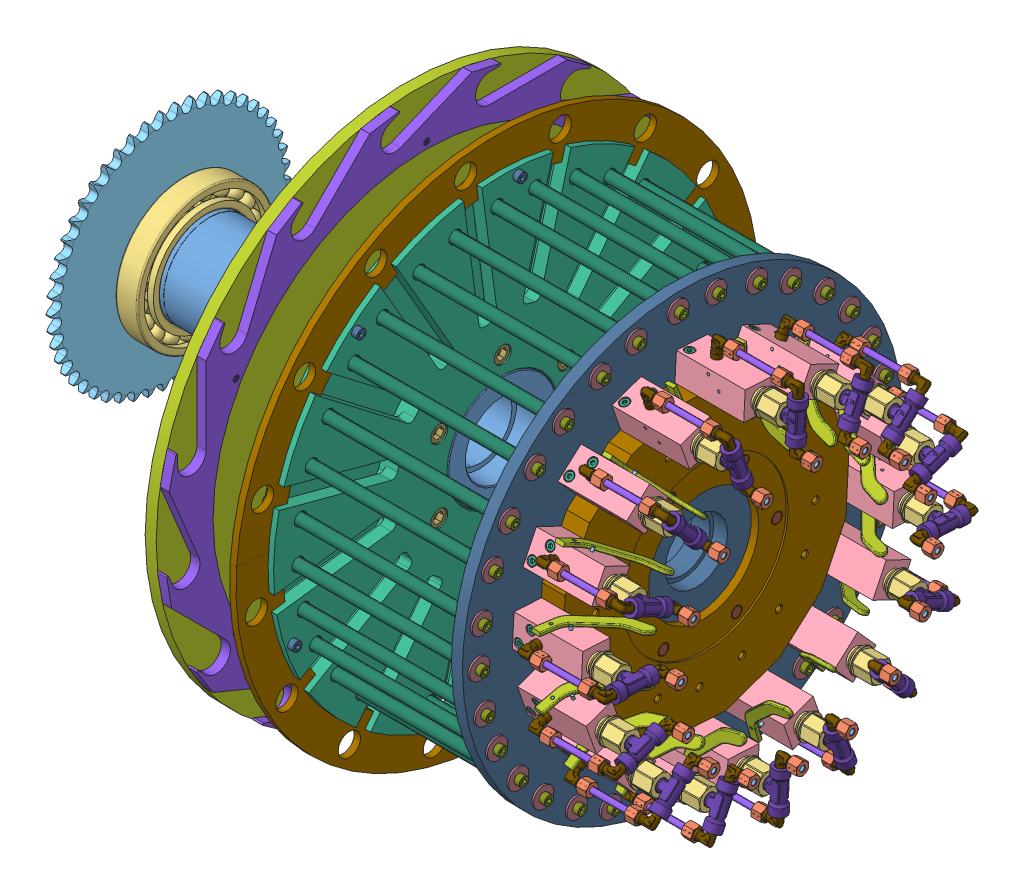
SolidWorks assembly assieme parte rotante, configuration Default. Lengths in mm.
Overall size (749.63 778.63 778.63).
555 component instances, 28 part files, 77 mates.
Components (placement in the parent):
- albero rotazione piatti-1: albero rotazione piatti [Default] at (60.413 18.3637 415) size (415 200 200)
- seger 100mm-1: seger 100mm [KS 1336 E - 100] at (-146.4567 18.3637 415) x (0 0 -1) z (1 0 0) size (107.55 112.98 3)
- SKF - 6020 - 20,DE,NC,20_68-1: SKF - 6020 - 20,DE,NC,20_68 [SKF - 6020 - 20,DE,NC,20_68] at (-131.4567 18.3637 415) x (1 0 0) z (0 -0.434476 -0.900684) size (24 150 150)
- calettatore d95-1: calettatore d95 [Default] at (-178.8867 18.3637 415) size (39.5 135 135)
- Chain wheel ISO - 50Z 10A-1-1: Chain wheel ISO - 50Z 10A-1 [Chain wheel ISO - 50Z 10A-1 --50SB120H25L95.0N] at (-164.8867 18.3637 415) size (25 262.06 262.51)
- Disco supporto montaggio e Colonne-1: Disco supporto montaggio e Colonne [Default] at (204.0433 18.3637 415) x (0 -0.866025 -0.5) z (1 0 0) size (499.6 499.6 29)
- SKF - 6020 - 20,DE,NC,20_68-2: SKF - 6020 - 20,DE,NC,20_68 [SKF - 6020 - 20,DE,NC,20_68] at (62.0433 18.3637 415) x (1 0 0) z (0 -0.432628 -0.901573) size (24 150 150)
- piatto rotante porta tappi-1: piatto rotante porta tappi [Default] at (99.0433 18.3637 415) x (0 0 -1) z (1 0 0) size (570 570 20.57)
- disco trasportatore tappi 31-1: disco trasportatore tappi 31 [Default] at (111.0433 18.3637 415) x (0 0.5 -0.866025) z (1 0 0) size (570 570 10.42)
- Distributore Rotante-1: Distributore Rotante [Default] at (425.0433 18.3637 415) x (0 -0.055301 -0.99847) z (1 0 0) size (310 310 25.54)
- disco trascinato porta distributore vuoto-1: disco trascinato porta distributore vuoto [Default] at (400.0433 18.3637 415) x (0 0.055301 0.99847) z (-1 0 0) size (480 480 50)
- m12 35mm-1: m12 35mm [ISO 4762 M12 x 35 - 35N] at (376.0433 -53.0243 378.8925) x (1 0 0) z (0 -0.5 0.866025) size (47 18 18)
- m12 90mm-3: m12 90mm [ISO 4762 M12 x 90 - 90N] at (203.0433 -21.6363 345.718) x (-1 0 0) z (0 -0.5 0.866025) size (102 18 18)
- rondella m6 22mm-1: rondella m6 22mm [Washer ISO 7094 - 6] at (99.0433 -101.6363 207.1539) x (1 0 0) z (0 -1 0) size (2 22 22)
- M6 20mm-1: M6 20mm [ISO 4762 M6 x 20 - 20N] at (91.0433 -101.6363 207.1539) x (1 0 0) z (0 0.5 0.866025) size (26 10 10)
- m12 35mm-2: m12 35mm [ISO 4762 M12 x 35 - 35N] at (376.0433 13.9397 335.1224) x (1 0 0) z (0 -1 0) size (47 18 18)
- m12 35mm-3: m12 35mm [ISO 4762 M12 x 35 - 35N] at (376.0433 85.3277 371.2299) x (1 0 0) z (0 -0.5 -0.866025) size (47 18 18)
- m12 35mm-4: m12 35mm [ISO 4762 M12 x 35 - 35N] at (376.0433 89.7517 451.1075) x (1 0 0) z (0 0.5 -0.866025) size (47 18 18)
- m12 35mm-5: m12 35mm [ISO 4762 M12 x 35 - 35N] at (376.0433 22.7877 494.8776) x (1 0 0) z (0 1 0) size (47 18 18)
- m12 35mm-6: m12 35mm [ISO 4762 M12 x 35 - 35N] at (376.0433 -48.6003 458.7701) x (1 0 0) z (0 0.5 0.866025) size (47 18 18)
- rondella m6 22mm-2: rondella m6 22mm [Washer ISO 7094 - 6] at (99.0433 138.3637 207.1539) x (1 0 0) z (0 -0.5 -0.866025) size (2 22 22)
- rondella m6 22mm-3: rondella m6 22mm [Washer ISO 7094 - 6] at (99.0433 258.3637 415) x (1 0 0) z (0 0.5 -0.866025) size (2 22 22)
- rondella m6 22mm-4: rondella m6 22mm [Washer ISO 7094 - 6] at (99.0433 138.3637 622.8461) x (1 0 0) z (0 1 0) size (2 22 22)
- rondella m6 22mm-5: rondella m6 22mm [Washer ISO 7094 - 6] at (99.0433 -101.6363 622.8461) x (1 0 0) z (0 0.5 0.866025) size (2 22 22)
- rondella m6 22mm-6: rondella m6 22mm [Washer ISO 7094 - 6] at (99.0433 -221.6363 415) x (1 0 0) z (0 -0.5 0.866025) size (2 22 22)
- M6 20mm-2: M6 20mm [ISO 4762 M6 x 20 - 20N] at (91.0433 138.3637 207.1539) x (1 0 0) z (0 -0.5 0.866025) size (26 10 10)
- M6 20mm-3: M6 20mm [ISO 4762 M6 x 20 - 20N] at (91.0433 258.3637 415) x (1 0 0) z (0 -1 0) size (26 10 10)
- M6 20mm-4: M6 20mm [ISO 4762 M6 x 20 - 20N] at (91.0433 138.3637 622.8461) x (1 0 0) z (0 -0.5 -0.866025) size (26 10 10)
- M6 20mm-5: M6 20mm [ISO 4762 M6 x 20 - 20N] at (91.0433 -101.6363 622.8461) x (1 0 0) z (0 0.5 -0.866025) size (26 10 10)
- M6 20mm-6: M6 20mm [ISO 4762 M6 x 20 - 20N] at (91.0433 -221.6363 415) x (1 0 0) z (0 1 0) size (26 10 10)
- m12 90mm-4: m12 90mm [ISO 4762 M12 x 90 - 90N] at (203.0433 58.3637 345.718) x (-1 0 0) z (0 -1 0) size (102 18 18)
- m12 90mm-5: m12 90mm [ISO 4762 M12 x 90 - 90N] at (203.0433 98.3637 415) x (-1 0 0) z (0 -0.5 -0.866025) size (102 18 18)
- m12 90mm-6: m12 90mm [ISO 4762 M12 x 90 - 90N] at (203.0433 58.3637 484.282) x (-1 0 0) z (0 0.5 -0.866025) size (102 18 18)
- m12 90mm-7: m12 90mm [ISO 4762 M12 x 90 - 90N] at (203.0433 -21.6363 484.282) x (-1 0 0) z (0 1 0) size (102 18 18)
- m12 90mm-8: m12 90mm [ISO 4762 M12 x 90 - 90N] at (203.0433 -61.6363 415) x (-1 0 0) z (0 0.5 0.866025) size (102 18 18)
- asta scorrimento carello-1: asta scorrimento carello [Default] at (287.5433 70.1437 197.9013) x (0 0 -1) z (1 0 0) size (12 12 225)
- rondella m6 22mm-7: rondella m6 22mm [Washer ISO 7094 - 6] at (175.0433 70.1437 197.9013) x (1 0 0) z (0 -1 0) size (2 22 22)
- M6 16mm-1: M6 16mm [ISO 4762 M6 x 16 - 16N] at (167.0433 70.1437 197.9013) size (22 10 10)
- M6 16mm-2: M6 16mm [ISO 4762 M6 x 16 - 16N] at (408.0433 70.1437 197.9013) x (-1 0 0) z (0 0 -1) size (22 10 10)
- rondella m6 22mm-8: rondella m6 22mm [Washer ISO 7094 - 6] at (400.0433 70.1437 197.9013) x (-1 0 0) z (0 1 0) size (2 22 22)
- rondella m6 22mm-9: rondella m6 22mm [Washer ISO 7094 - 6] at (175.0433 24.5373 191.8971) x (1 0 0) z (0 -0.965926 -0.258819) size (2 22 22)
- M6 16mm-3: M6 16mm [ISO 4762 M6 x 16 - 16N] at (167.0433 24.5373 191.8971) x (1 0 0) z (0 0.258819 -0.965926) size (22 10 10)
- asta scorrimento carello-2: asta scorrimento carello [Default] at (287.5433 24.5373 191.8971) x (0 0.258819 -0.965926) z (-1 0 0) size (12 12 225)
- rondella m6 22mm-10: rondella m6 22mm [Washer ISO 7094 - 6] at (400.0433 24.5373 191.8971) x (-1 0 0) z (0 0.965926 0.258819) size (2 22 22)
- M6 16mm-4: M6 16mm [ISO 4762 M6 x 16 - 16N] at (408.0433 24.5373 191.8971) x (-1 0 0) z (0 -0.258819 0.965926) size (22 10 10)
- AssiemeValvola-1: AssiemeValvola [Default] at (515.3257 74.6348 254.5832) x (0 -0.331007 0.943628) z (0 0.943628 0.331007) size (90.26 138.63 38)
  - RaccordoT-1: RaccordoT [Default] at origin size (43 29.75 16.5)
  - Raccordo a L-1: Raccordo a L [Default] at (-30 0 0) x (0 -1 0) z (0 0 -1) size (28.34 25.51 14.01)
    - 1809_06_10_01-1: 1809_06_10_01 [Default] at origin size (22.49 23 10)
    - 1809_06_10_02-1: 1809_06_10_02 [Default] at origin size (6.5 8.5 8.5)
    - 1809_06_10_03-1: 1809_06_10_03 [Default] at origin size (11.02 15.01 14.01)
  - Raccordo a L-2: Raccordo a L [Default] at (30 0 0) x (0 1 0) z (0 0 -1) size (28.34 25.51 14.01)
    - 1809_06_10_01-1: 1809_06_10_01 [Default] at origin size (22.49 23 10)
    - 1809_06_10_02-1: 1809_06_10_02 [Default] at origin size (6.5 8.5 8.5)
    - 1809_06_10_03-1: 1809_06_10_03 [Default] at origin size (11.02 15.01 14.01)
  - TappoChiusura-1: TappoChiusura [Default] at (0 -32 0) x (0 -1 0) z (0 0 1) size (38.28 26.74 26.74)
  - CorpoValvola-1: CorpoValvola [Default] at (-15 -115.2824 0) size (30 75 34)
  - Raccordo a L-3: Raccordo a L [Default] at (-30 -88.2824 0) x (0 1 0) z (0 0 1) size (28.34 25.51 14.01)
    - 1809_06_10_01-1: 1809_06_10_01 [Default] at origin size (22.49 23 10)
    - 1809_06_10_02-1: 1809_06_10_02 [Default] at origin size (6.5 8.5 8.5)
    - 1809_06_10_03-1: 1809_06_10_03 [Default] at origin size (11.02 15.01 14.01)
  - Spina_3x38-1: Spina_3x38 [Default] at (0 -68.2824 -21) x (-1 0 0) z (0 0 1) size (3 3 38)
  - Spina_3x38-2: Spina_3x38 [Default] at (-10 -80.2824 -21) x (0.996193 0.087174 0) z (0 0 1) size (3 3 38)
  - M5 40mm-3: M5 40mm [ISO 4762 M5 x 40 - 40N] at (-14.6 -108.7824 9) size (45 8.5 8.5)
  - M5 40mm-2: M5 40mm [ISO 4762 M5 x 40 - 40N] at (-14.6 -96.7824 -9) size (45 8.5 8.5)
  - LevaValvola-1: LevaValvola [Default] at (-24.507 -86.571 -17) x (0.996193 0.087174 0) z (0 0 1) size (77.55 60.2 4)
  - Tubo-1: Tubo [Default] at (-30 -15.9665 0) x (1 0 0) z (0 -1 0) size (6 6 56.4)
- M6 16mm-5: M6 16mm [ISO 4762 M6 x 16 - 16N] at (167.0433 -16.8778 194.6116) x (1 0 0) z (0 0.382683 0.92388) size (22 10 10)
- M6 16mm-6: M6 16mm [ISO 4762 M6 x 16 - 16N] at (167.0433 -98.5342 224.874) x (1 0 0) z (0 0.707107 0.707107) size (22 10 10)
- M6 16mm-7: M6 16mm [ISO 4762 M6 x 16 - 16N] at (167.0433 -162.3939 284.0814) x (1 0 0) z (0 0.92388 0.382683) size (22 10 10)
- M6 16mm-8: M6 16mm [ISO 4762 M6 x 16 - 16N] at (167.0433 -198.735 363.22) x (1 0 0) z (0 1 0) size (22 10 10)
- M6 16mm-9: M6 16mm [ISO 4762 M6 x 16 - 16N] at (167.0433 -202.0247 450.2415) x (1 0 0) z (0 0.92388 -0.382683) size (22 10 10)
- M6 16mm-10: M6 16mm [ISO 4762 M6 x 16 - 16N] at (167.0433 -171.7623 531.8979) x (1 0 0) z (0 0.707107 -0.707107) size (22 10 10)
- M6 16mm-11: M6 16mm [ISO 4762 M6 x 16 - 16N] at (167.0433 -112.5549 595.7576) x (1 0 0) z (0 0.382683 -0.92388) size (22 10 10)
- M6 16mm-12: M6 16mm [ISO 4762 M6 x 16 - 16N] at (167.0433 -33.4163 632.0987) x (1 0 0) z (0 0 -1) size (22 10 10)
- M6 16mm-13: M6 16mm [ISO 4762 M6 x 16 - 16N] at (167.0433 53.6052 635.3884) x (1 0 0) z (0 -0.382683 -0.92388) size (22 10 10)
- M6 16mm-14: M6 16mm [ISO 4762 M6 x 16 - 16N] at (167.0433 135.2616 605.126) x (1 0 0) z (0 -0.707107 -0.707107) size (22 10 10)
- M6 16mm-15: M6 16mm [ISO 4762 M6 x 16 - 16N] at (167.0433 199.1213 545.9186) x (1 0 0) z (0 -0.92388 -0.382683) size (22 10 10)
- M6 16mm-16: M6 16mm [ISO 4762 M6 x 16 - 16N] at (167.0433 235.4624 466.78) x (1 0 0) z (0 -1 0) size (22 10 10)
- M6 16mm-17: M6 16mm [ISO 4762 M6 x 16 - 16N] at (167.0433 238.7521 379.7585) x (1 0 0) z (0 -0.92388 0.382683) size (22 10 10)
- M6 16mm-18: M6 16mm [ISO 4762 M6 x 16 - 16N] at (167.0433 208.4897 298.1021) x (1 0 0) z (0 -0.707107 0.707107) size (22 10 10)
- M6 16mm-19: M6 16mm [ISO 4762 M6 x 16 - 16N] at (167.0433 149.2823 234.2424) x (1 0 0) z (0 -0.382683 0.92388) size (22 10 10)
- rondella m6 22mm-11: rondella m6 22mm [Washer ISO 7094 - 6] at (175.0433 -16.8778 194.6116) x (1 0 0) z (0 -0.92388 0.382683) size (2 22 22)
- rondella m6 22mm-12: rondella m6 22mm [Washer ISO 7094 - 6] at (175.0433 -98.5342 224.874) x (1 0 0) z (0 -0.707107 0.707107) size (2 22 22)
- rondella m6 22mm-13: rondella m6 22mm [Washer ISO 7094 - 6] at (175.0433 -162.3939 284.0814) x (1 0 0) z (0 -0.382683 0.92388) size (2 22 22)
- rondella m6 22mm-14: rondella m6 22mm [Washer ISO 7094 - 6] at (175.0433 -198.735 363.22) size (2 22 22)
- rondella m6 22mm-15: rondella m6 22mm [Washer ISO 7094 - 6] at (175.0433 -202.0247 450.2415) x (1 0 0) z (0 0.382683 0.92388) size (2 22 22)
- rondella m6 22mm-16: rondella m6 22mm [Washer ISO 7094 - 6] at (175.0433 -171.7623 531.8979) x (1 0 0) z (0 0.707107 0.707107) size (2 22 22)
- rondella m6 22mm-17: rondella m6 22mm [Washer ISO 7094 - 6] at (175.0433 -112.5549 595.7576) x (1 0 0) z (0 0.92388 0.382683) size (2 22 22)
- rondella m6 22mm-18: rondella m6 22mm [Washer ISO 7094 - 6] at (175.0433 -33.4163 632.0987) x (1 0 0) z (0 1 0) size (2 22 22)
- rondella m6 22mm-19: rondella m6 22mm [Washer ISO 7094 - 6] at (175.0433 53.6052 635.3884) x (1 0 0) z (0 0.92388 -0.382683) size (2 22 22)
- rondella m6 22mm-20: rondella m6 22mm [Washer ISO 7094 - 6] at (175.0433 135.2616 605.126) x (1 0 0) z (0 0.707107 -0.707107) size (2 22 22)
- rondella m6 22mm-21: rondella m6 22mm [Washer ISO 7094 - 6] at (175.0433 199.1213 545.9186) x (1 0 0) z (0 0.382683 -0.92388) size (2 22 22)
- rondella m6 22mm-22: rondella m6 22mm [Washer ISO 7094 - 6] at (175.0433 235.4624 466.78) x (1 0 0) z (0 0 -1) size (2 22 22)
- rondella m6 22mm-23: rondella m6 22mm [Washer ISO 7094 - 6] at (175.0433 238.7521 379.7585) x (1 0 0) z (0 -0.382683 -0.92388) size (2 22 22)
- rondella m6 22mm-24: rondella m6 22mm [Washer ISO 7094 - 6] at (175.0433 208.4897 298.1021) x (1 0 0) z (0 -0.707107 -0.707107) size (2 22 22)
- rondella m6 22mm-25: rondella m6 22mm [Washer ISO 7094 - 6] at (175.0433 149.2823 234.2424) x (1 0 0) z (0 -0.92388 -0.382683) size (2 22 22)
- asta scorrimento carello-3: asta scorrimento carello [Default] at (287.5433 -16.8778 194.6116) x (0 -0.382683 -0.92388) z (1 0 0) size (12 12 225)
- asta scorrimento carello-4: asta scorrimento carello [Default] at (287.5433 -98.5342 224.874) x (0 -0.707107 -0.707107) z (1 0 0) size (12 12 225)
- asta scorrimento carello-5: asta scorrimento carello [Default] at (287.5433 -162.3939 284.0814) x (0 -0.92388 -0.382683) z (1 0 0) size (12 12 225)
- asta scorrimento carello-6: asta scorrimento carello [Default] at (287.5433 -198.735 363.22) x (0 -1 0) z (1 0 0) size (12 12 225)
- asta scorrimento carello-7: asta scorrimento carello [Default] at (287.5433 -202.0247 450.2415) x (0 -0.92388 0.382683) z (1 0 0) size (12 12 225)
- asta scorrimento carello-8: asta scorrimento carello [Default] at (287.5433 -171.7623 531.8979) x (0 -0.707107 0.707107) z (1 0 0) size (12 12 225)
- asta scorrimento carello-9: asta scorrimento carello [Default] at (287.5433 -112.5549 595.7576) x (0 -0.382683 0.92388) z (1 0 0) size (12 12 225)
- asta scorrimento carello-10: asta scorrimento carello [Default] at (287.5433 -33.4163 632.0987) x (0 0 1) z (1 0 0) size (12 12 225)
- asta scorrimento carello-11: asta scorrimento carello [Default] at (287.5433 53.6052 635.3884) x (0 0.382683 0.92388) z (1 0 0) size (12 12 225)
- asta scorrimento carello-12: asta scorrimento carello [Default] at (287.5433 135.2616 605.126) x (0 0.707107 0.707107) z (1 0 0) size (12 12 225)
- asta scorrimento carello-13: asta scorrimento carello [Default] at (287.5433 199.1213 545.9186) x (0 0.92388 0.382683) z (1 0 0) size (12 12 225)
- asta scorrimento carello-14: asta scorrimento carello [Default] at (287.5433 235.4624 466.78) x (0 1 0) z (1 0 0) size (12 12 225)
- asta scorrimento carello-15: asta scorrimento carello [Default] at (287.5433 238.7521 379.7585) x (0 0.92388 -0.382683) z (1 0 0) size (12 12 225)
- asta scorrimento carello-16: asta scorrimento carello [Default] at (287.5433 208.4897 298.1021) x (0 0.707107 -0.707107) z (1 0 0) size (12 12 225)
- asta scorrimento carello-17: asta scorrimento carello [Default] at (287.5433 149.2823 234.2424) x (0 0.382683 -0.92388) z (1 0 0) size (12 12 225)
- M6 16mm-20: M6 16mm [ISO 4762 M6 x 16 - 16N] at (408.0433 -16.8778 194.6116) x (-1 0 0) z (0 -0.382683 -0.92388) size (22 10 10)
- M6 16mm-21: M6 16mm [ISO 4762 M6 x 16 - 16N] at (408.0433 -98.5342 224.874) x (-1 0 0) z (0 -0.707107 -0.707107) size (22 10 10)
- M6 16mm-22: M6 16mm [ISO 4762 M6 x 16 - 16N] at (408.0433 -162.3939 284.0814) x (-1 0 0) z (0 -0.92388 -0.382683) size (22 10 10)
- M6 16mm-23: M6 16mm [ISO 4762 M6 x 16 - 16N] at (408.0433 -198.735 363.22) x (-1 0 0) z (0 -1 0) size (22 10 10)
- M6 16mm-24: M6 16mm [ISO 4762 M6 x 16 - 16N] at (408.0433 -202.0247 450.2415) x (-1 0 0) z (0 -0.92388 0.382683) size (22 10 10)
- M6 16mm-25: M6 16mm [ISO 4762 M6 x 16 - 16N] at (408.0433 -171.7623 531.8979) x (-1 0 0) z (0 -0.707107 0.707107) size (22 10 10)
- M6 16mm-26: M6 16mm [ISO 4762 M6 x 16 - 16N] at (408.0433 -112.5549 595.7576) x (-1 0 0) z (0 -0.382683 0.92388) size (22 10 10)
- M6 16mm-27: M6 16mm [ISO 4762 M6 x 16 - 16N] at (408.0433 -33.4163 632.0987) x (-1 0 0) z (0 0 1) size (22 10 10)
- M6 16mm-28: M6 16mm [ISO 4762 M6 x 16 - 16N] at (408.0433 53.6052 635.3884) x (-1 0 0) z (0 0.382683 0.92388) size (22 10 10)
- M6 16mm-29: M6 16mm [ISO 4762 M6 x 16 - 16N] at (408.0433 135.2616 605.126) x (-1 0 0) z (0 0.707107 0.707107) size (22 10 10)
- M6 16mm-30: M6 16mm [ISO 4762 M6 x 16 - 16N] at (408.0433 199.1213 545.9186) x (-1 0 0) z (0 0.92388 0.382683) size (22 10 10)
- M6 16mm-31: M6 16mm [ISO 4762 M6 x 16 - 16N] at (408.0433 235.4624 466.78) x (-1 0 0) z (0 1 0) size (22 10 10)
- M6 16mm-32: M6 16mm [ISO 4762 M6 x 16 - 16N] at (408.0433 238.7521 379.7585) x (-1 0 0) z (0 0.92388 -0.382683) size (22 10 10)
- M6 16mm-33: M6 16mm [ISO 4762 M6 x 16 - 16N] at (408.0433 208.4897 298.1021) x (-1 0 0) z (0 0.707107 -0.707107) size (22 10 10)
- M6 16mm-34: M6 16mm [ISO 4762 M6 x 16 - 16N] at (408.0433 149.2823 234.2424) x (-1 0 0) z (0 0.382683 -0.92388) size (22 10 10)
- rondella m6 22mm-26: rondella m6 22mm [Washer ISO 7094 - 6] at (400.0433 -16.8778 194.6116) x (-1 0 0) z (0 0.92388 -0.382683) size (2 22 22)
- rondella m6 22mm-27: rondella m6 22mm [Washer ISO 7094 - 6] at (400.0433 -98.5342 224.874) x (-1 0 0) z (0 0.707107 -0.707107) size (2 22 22)
- rondella m6 22mm-28: rondella m6 22mm [Washer ISO 7094 - 6] at (400.0433 -162.3939 284.0814) x (-1 0 0) z (0 0.382683 -0.92388) size (2 22 22)
- rondella m6 22mm-29: rondella m6 22mm [Washer ISO 7094 - 6] at (400.0433 -198.735 363.22) x (-1 0 0) z (0 0 -1) size (2 22 22)
- rondella m6 22mm-30: rondella m6 22mm [Washer ISO 7094 - 6] at (400.0433 -202.0247 450.2415) x (-1 0 0) z (0 -0.382683 -0.92388) size (2 22 22)
- rondella m6 22mm-31: rondella m6 22mm [Washer ISO 7094 - 6] at (400.0433 -171.7623 531.8979) x (-1 0 0) z (0 -0.707107 -0.707107) size (2 22 22)
- rondella m6 22mm-32: rondella m6 22mm [Washer ISO 7094 - 6] at (400.0433 -112.5549 595.7576) x (-1 0 0) z (0 -0.92388 -0.382683) size (2 22 22)
- rondella m6 22mm-33: rondella m6 22mm [Washer ISO 7094 - 6] at (400.0433 -33.4163 632.0987) x (-1 0 0) z (0 -1 0) size (2 22 22)
- rondella m6 22mm-34: rondella m6 22mm [Washer ISO 7094 - 6] at (400.0433 53.6052 635.3884) x (-1 0 0) z (0 -0.92388 0.382683) size (2 22 22)
- rondella m6 22mm-35: rondella m6 22mm [Washer ISO 7094 - 6] at (400.0433 135.2616 605.126) x (-1 0 0) z (0 -0.707107 0.707107) size (2 22 22)
- rondella m6 22mm-36: rondella m6 22mm [Washer ISO 7094 - 6] at (400.0433 199.1213 545.9186) x (-1 0 0) z (0 -0.382683 0.92388) size (2 22 22)
- rondella m6 22mm-37: rondella m6 22mm [Washer ISO 7094 - 6] at (400.0433 235.4624 466.78) x (-1 0 0) z (0 0 1) size (2 22 22)
- rondella m6 22mm-38: rondella m6 22mm [Washer ISO 7094 - 6] at (400.0433 238.7521 379.7585) x (-1 0 0) z (0 0.382683 0.92388) size (2 22 22)
- rondella m6 22mm-39: rondella m6 22mm [Washer ISO 7094 - 6] at (400.0433 208.4897 298.1021) x (-1 0 0) z (0 0.707107 0.707107) size (2 22 22)
- rondella m6 22mm-40: rondella m6 22mm [Washer ISO 7094 - 6] at (400.0433 149.2823 234.2424) x (-1 0 0) z (0 0.92388 0.382683) size (2 22 22)
- rondella m6 22mm-41: rondella m6 22mm [Washer ISO 7094 - 6] at (175.0433 -61.3104 206.5173) x (1 0 0) z (0 -0.991445 0.130526) size (2 22 22)
- rondella m6 22mm-42: rondella m6 22mm [Washer ISO 7094 - 6] at (175.0433 -135.0285 252.8771) x (1 0 0) z (0 -0.866025 0.5) size (2 22 22)
- rondella m6 22mm-43: rondella m6 22mm [Washer ISO 7094 - 6] at (175.0433 -185.3939 323.9186) x (1 0 0) z (0 -0.608761 0.793353) size (2 22 22)
- rondella m6 22mm-44: rondella m6 22mm [Washer ISO 7094 - 6] at (175.0433 -204.7392 408.8264) x (1 0 0) z (0 -0.258819 0.965926) size (2 22 22)
- rondella m6 22mm-45: rondella m6 22mm [Washer ISO 7094 - 6] at (175.0433 -190.119 494.6741) x (1 0 0) z (0 0.130526 0.991445) size (2 22 22)
- rondella m6 22mm-46: rondella m6 22mm [Washer ISO 7094 - 6] at (175.0433 -143.7592 568.3922) x (1 0 0) z (0 0.5 0.866025) size (2 22 22)
- rondella m6 22mm-47: rondella m6 22mm [Washer ISO 7094 - 6] at (175.0433 -72.7177 618.7576) x (1 0 0) z (0 0.793353 0.608761) size (2 22 22)
- rondella m6 22mm-48: rondella m6 22mm [Washer ISO 7094 - 6] at (175.0433 12.1901 638.1029) x (1 0 0) z (0 0.965926 0.258819) size (2 22 22)
- rondella m6 22mm-49: rondella m6 22mm [Washer ISO 7094 - 6] at (175.0433 98.0378 623.4827) x (1 0 0) z (0 0.991445 -0.130526) size (2 22 22)
- rondella m6 22mm-50: rondella m6 22mm [Washer ISO 7094 - 6] at (175.0433 171.7559 577.1229) x (1 0 0) z (0 0.866025 -0.5) size (2 22 22)
- rondella m6 22mm-51: rondella m6 22mm [Washer ISO 7094 - 6] at (175.0433 222.1213 506.0814) x (1 0 0) z (0 0.608761 -0.793353) size (2 22 22)
- rondella m6 22mm-52: rondella m6 22mm [Washer ISO 7094 - 6] at (175.0433 241.4666 421.1736) x (1 0 0) z (0 0.258819 -0.965926) size (2 22 22)
- rondella m6 22mm-53: rondella m6 22mm [Washer ISO 7094 - 6] at (175.0433 226.8464 335.3259) x (1 0 0) z (0 -0.130526 -0.991445) size (2 22 22)
- rondella m6 22mm-54: rondella m6 22mm [Washer ISO 7094 - 6] at (175.0433 180.4866 261.6078) x (1 0 0) z (0 -0.5 -0.866025) size (2 22 22)
- rondella m6 22mm-55: rondella m6 22mm [Washer ISO 7094 - 6] at (175.0433 109.4451 211.2424) x (1 0 0) z (0 -0.793353 -0.608761) size (2 22 22)
- M6 16mm-35: M6 16mm [ISO 4762 M6 x 16 - 16N] at (167.0433 -61.3104 206.5173) x (1 0 0) z (0 -0.130526 -0.991445) size (22 10 10)
- M6 16mm-36: M6 16mm [ISO 4762 M6 x 16 - 16N] at (167.0433 -135.0285 252.8771) x (1 0 0) z (0 -0.5 -0.866025) size (22 10 10)
- M6 16mm-37: M6 16mm [ISO 4762 M6 x 16 - 16N] at (167.0433 -185.3939 323.9186) x (1 0 0) z (0 -0.793353 -0.608761) size (22 10 10)
- M6 16mm-38: M6 16mm [ISO 4762 M6 x 16 - 16N] at (167.0433 -204.7392 408.8264) x (1 0 0) z (0 -0.965926 -0.258819) size (22 10 10)
- M6 16mm-39: M6 16mm [ISO 4762 M6 x 16 - 16N] at (167.0433 -190.119 494.6741) x (1 0 0) z (0 -0.991445 0.130526) size (22 10 10)
- M6 16mm-40: M6 16mm [ISO 4762 M6 x 16 - 16N] at (167.0433 -143.7592 568.3922) x (1 0 0) z (0 -0.866025 0.5) size (22 10 10)
- M6 16mm-41: M6 16mm [ISO 4762 M6 x 16 - 16N] at (167.0433 -72.7177 618.7576) x (1 0 0) z (0 -0.608761 0.793353) size (22 10 10)
- M6 16mm-42: M6 16mm [ISO 4762 M6 x 16 - 16N] at (167.0433 12.1901 638.1029) x (1 0 0) z (0 -0.258819 0.965926) size (22 10 10)
- M6 16mm-43: M6 16mm [ISO 4762 M6 x 16 - 16N] at (167.0433 98.0378 623.4827) x (1 0 0) z (0 0.130526 0.991445) size (22 10 10)
- M6 16mm-44: M6 16mm [ISO 4762 M6 x 16 - 16N] at (167.0433 171.7559 577.1229) x (1 0 0) z (0 0.5 0.866025) size (22 10 10)
- M6 16mm-45: M6 16mm [ISO 4762 M6 x 16 - 16N] at (167.0433 222.1213 506.0814) x (1 0 0) z (0 0.793353 0.608761) size (22 10 10)
- M6 16mm-46: M6 16mm [ISO 4762 M6 x 16 - 16N] at (167.0433 241.4666 421.1736) x (1 0 0) z (0 0.965926 0.258819) size (22 10 10)
- M6 16mm-47: M6 16mm [ISO 4762 M6 x 16 - 16N] at (167.0433 226.8464 335.3259) x (1 0 0) z (0 0.991445 -0.130526) size (22 10 10)
- M6 16mm-48: M6 16mm [ISO 4762 M6 x 16 - 16N] at (167.0433 180.4866 261.6078) x (1 0 0) z (0 0.866025 -0.5) size (22 10 10)
- M6 16mm-49: M6 16mm [ISO 4762 M6 x 16 - 16N] at (167.0433 109.4451 211.2424) x (1 0 0) z (0 0.608761 -0.793353) size (22 10 10)
- asta scorrimento carello-18: asta scorrimento carello [Default] at (287.5433 -61.3104 206.5173) x (0 -0.130526 -0.991445) z (-1 0 0) size (12 12 225)
- asta scorrimento carello-19: asta scorrimento carello [Default] at (287.5433 -135.0285 252.8771) x (0 -0.5 -0.866025) z (-1 0 0) size (12 12 225)
- asta scorrimento carello-20: asta scorrimento carello [Default] at (287.5433 -185.3939 323.9186) x (0 -0.793353 -0.608761) z (-1 0 0) size (12 12 225)
- asta scorrimento carello-21: asta scorrimento carello [Default] at (287.5433 -204.7392 408.8264) x (0 -0.965926 -0.258819) z (-1 0 0) size (12 12 225)
- asta scorrimento carello-22: asta scorrimento carello [Default] at (287.5433 -190.119 494.6741) x (0 -0.991445 0.130526) z (-1 0 0) size (12 12 225)
- asta scorrimento carello-23: asta scorrimento carello [Default] at (287.5433 -143.7592 568.3922) x (0 -0.866025 0.5) z (-1 0 0) size (12 12 225)
- asta scorrimento carello-24: asta scorrimento carello [Default] at (287.5433 -72.7177 618.7576) x (0 -0.608761 0.793353) z (-1 0 0) size (12 12 225)
- asta scorrimento carello-25: asta scorrimento carello [Default] at (287.5433 12.1901 638.1029) x (0 -0.258819 0.965926) z (-1 0 0) size (12 12 225)
- asta scorrimento carello-26: asta scorrimento carello [Default] at (287.5433 98.0378 623.4827) x (0 0.130526 0.991445) z (-1 0 0) size (12 12 225)
- asta scorrimento carello-27: asta scorrimento carello [Default] at (287.5433 171.7559 577.1229) x (0 0.5 0.866025) z (-1 0 0) size (12 12 225)
- asta scorrimento carello-28: asta scorrimento carello [Default] at (287.5433 222.1213 506.0814) x (0 0.793353 0.608761) z (-1 0 0) size (12 12 225)
- asta scorrimento carello-29: asta scorrimento carello [Default] at (287.5433 241.4666 421.1736) x (0 0.965926 0.258819) z (-1 0 0) size (12 12 225)
- asta scorrimento carello-30: asta scorrimento carello [Default] at (287.5433 226.8464 335.3259) x (0 0.991445 -0.130526) z (-1 0 0) size (12 12 225)
- asta scorrimento carello-31: asta scorrimento carello [Default] at (287.5433 180.4866 261.6078) x (0 0.866025 -0.5) z (-1 0 0) size (12 12 225)
- asta scorrimento carello-32: asta scorrimento carello [Default] at (287.5433 109.4451 211.2424) x (0 0.608761 -0.793353) z (-1 0 0) size (12 12 225)
- rondella m6 22mm-56: rondella m6 22mm [Washer ISO 7094 - 6] at (400.0433 -61.3104 206.5173) x (-1 0 0) z (0 0.991445 -0.130526) size (2 22 22)
- rondella m6 22mm-57: rondella m6 22mm [Washer ISO 7094 - 6] at (400.0433 -135.0285 252.8771) x (-1 0 0) z (0 0.866025 -0.5) size (2 22 22)
- rondella m6 22mm-58: rondella m6 22mm [Washer ISO 7094 - 6] at (400.0433 -185.3939 323.9186) x (-1 0 0) z (0 0.608761 -0.793353) size (2 22 22)
- rondella m6 22mm-59: rondella m6 22mm [Washer ISO 7094 - 6] at (400.0433 -204.7392 408.8264) x (-1 0 0) z (0 0.258819 -0.965926) size (2 22 22)
- rondella m6 22mm-60: rondella m6 22mm [Washer ISO 7094 - 6] at (400.0433 -190.119 494.6741) x (-1 0 0) z (0 -0.130526 -0.991445) size (2 22 22)
- rondella m6 22mm-61: rondella m6 22mm [Washer ISO 7094 - 6] at (400.0433 -143.7592 568.3922) x (-1 0 0) z (0 -0.5 -0.866025) size (2 22 22)
- rondella m6 22mm-62: rondella m6 22mm [Washer ISO 7094 - 6] at (400.0433 -72.7177 618.7576) x (-1 0 0) z (0 -0.793353 -0.608761) size (2 22 22)
- rondella m6 22mm-63: rondella m6 22mm [Washer ISO 7094 - 6] at (400.0433 12.1901 638.1029) x (-1 0 0) z (0 -0.965926 -0.258819) size (2 22 22)
- rondella m6 22mm-64: rondella m6 22mm [Washer ISO 7094 - 6] at (400.0433 98.0378 623.4827) x (-1 0 0) z (0 -0.991445 0.130526) size (2 22 22)
- rondella m6 22mm-65: rondella m6 22mm [Washer ISO 7094 - 6] at (400.0433 171.7559 577.1229) x (-1 0 0) z (0 -0.866025 0.5) size (2 22 22)
- rondella m6 22mm-66: rondella m6 22mm [Washer ISO 7094 - 6] at (400.0433 222.1213 506.0814) x (-1 0 0) z (0 -0.608761 0.793353) size (2 22 22)
- rondella m6 22mm-67: rondella m6 22mm [Washer ISO 7094 - 6] at (400.0433 241.4666 421.1736) x (-1 0 0) z (0 -0.258819 0.965926) size (2 22 22)
- rondella m6 22mm-68: rondella m6 22mm [Washer ISO 7094 - 6] at (400.0433 226.8464 335.3259) x (-1 0 0) z (0 0.130526 0.991445) size (2 22 22)
- rondella m6 22mm-69: rondella m6 22mm [Washer ISO 7094 - 6] at (400.0433 180.4866 261.6078) x (-1 0 0) z (0 0.5 0.866025) size (2 22 22)
- rondella m6 22mm-70: rondella m6 22mm [Washer ISO 7094 - 6] at (400.0433 109.4451 211.2424) x (-1 0 0) z (0 0.793353 0.608761) size (2 22 22)
- M6 16mm-50: M6 16mm [ISO 4762 M6 x 16 - 16N] at (408.0433 -61.3104 206.5173) x (-1 0 0) z (0 0.130526 0.991445) size (22 10 10)
- M6 16mm-51: M6 16mm [ISO 4762 M6 x 16 - 16N] at (408.0433 -135.0285 252.8771) x (-1 0 0) z (0 0.5 0.866025) size (22 10 10)
- M6 16mm-52: M6 16mm [ISO 4762 M6 x 16 - 16N] at (408.0433 -185.3939 323.9186) x (-1 0 0) z (0 0.793353 0.608761) size (22 10 10)
- M6 16mm-53: M6 16mm [ISO 4762 M6 x 16 - 16N] at (408.0433 -204.7392 408.8264) x (-1 0 0) z (0 0.965926 0.258819) size (22 10 10)
- M6 16mm-54: M6 16mm [ISO 4762 M6 x 16 - 16N] at (408.0433 -190.119 494.6741) x (-1 0 0) z (0 0.991445 -0.130526) size (22 10 10)
- M6 16mm-55: M6 16mm [ISO 4762 M6 x 16 - 16N] at (408.0433 -143.7592 568.3922) x (-1 0 0) z (0 0.866025 -0.5) size (22 10 10)
- M6 16mm-56: M6 16mm [ISO 4762 M6 x 16 - 16N] at (408.0433 -72.7177 618.7576) x (-1 0 0) z (0 0.608761 -0.793353) size (22 10 10)
- M6 16mm-57: M6 16mm [ISO 4762 M6 x 16 - 16N] at (408.0433 12.1901 638.1029) x (-1 0 0) z (0 0.258819 -0.965926) size (22 10 10)
- M6 16mm-58: M6 16mm [ISO 4762 M6 x 16 - 16N] at (408.0433 98.0378 623.4827) x (-1 0 0) z (0 -0.130526 -0.991445) size (22 10 10)
- M6 16mm-59: M6 16mm [ISO 4762 M6 x 16 - 16N] at (408.0433 171.7559 577.1229) x (-1 0 0) z (0 -0.5 -0.866025) size (22 10 10)
- M6 16mm-60: M6 16mm [ISO 4762 M6 x 16 - 16N] at (408.0433 222.1213 506.0814) x (-1 0 0) z (0 -0.793353 -0.608761) size (22 10 10)
- M6 16mm-61: M6 16mm [ISO 4762 M6 x 16 - 16N] at (408.0433 241.4666 421.1736) x (-1 0 0) z (0 -0.965926 -0.258819) size (22 10 10)
- M6 16mm-62: M6 16mm [ISO 4762 M6 x 16 - 16N] at (408.0433 226.8464 335.3259) x (-1 0 0) z (0 -0.991445 0.130526) size (22 10 10)
- M6 16mm-63: M6 16mm [ISO 4762 M6 x 16 - 16N] at (408.0433 180.4866 261.6078) x (-1 0 0) z (0 -0.866025 0.5) size (22 10 10)
- M6 16mm-64: M6 16mm [ISO 4762 M6 x 16 - 16N] at (408.0433 109.4451 211.2424) x (-1 0 0) z (0 -0.608761 0.793353) size (22 10 10)
- AssiemeValvola-2: AssiemeValvola [Default] at (515.3257 8.9626 245.2601) x (0 0.055301 0.99847) z (0 0.99847 -0.055301) size (90.26 138.63 38)
  - RaccordoT-1: RaccordoT [Default] at origin size (43 29.75 16.5)
  - Raccordo a L-1: Raccordo a L [Default] at (-30 0 0) x (0 -1 0) z (0 0 -1) size (28.34 25.51 14.01)
    - 1809_06_10_01-1: 1809_06_10_01 [Default] at origin size (22.49 23 10)
    - 1809_06_10_02-1: 1809_06_10_02 [Default] at origin size (6.5 8.5 8.5)
    - 1809_06_10_03-1: 1809_06_10_03 [Default] at origin size (11.02 15.01 14.01)
  - Raccordo a L-2: Raccordo a L [Default] at (30 0 0) x (0 1 0) z (0 0 -1) size (28.34 25.51 14.01)
    - 1809_06_10_01-1: 1809_06_10_01 [Default] at origin size (22.49 23 10)
    - 1809_06_10_02-1: 1809_06_10_02 [Default] at origin size (6.5 8.5 8.5)
    - 1809_06_10_03-1: 1809_06_10_03 [Default] at origin size (11.02 15.01 14.01)
  - TappoChiusura-1: TappoChiusura [Default] at (0 -32 0) x (0 -1 0) z (0 0 1) size (38.28 26.74 26.74)
  - CorpoValvola-1: CorpoValvola [Default] at (-15 -115.2824 0) size (30 75 34)
  - Raccordo a L-3: Raccordo a L [Default] at (-30 -88.2824 0) x (0 1 0) z (0 0 1) size (28.34 25.51 14.01)
    - 1809_06_10_01-1: 1809_06_10_01 [Default] at origin size (22.49 23 10)
    - 1809_06_10_02-1: 1809_06_10_02 [Default] at origin size (6.5 8.5 8.5)
    - 1809_06_10_03-1: 1809_06_10_03 [Default] at origin size (11.02 15.01 14.01)
  - Spina_3x38-1: Spina_3x38 [Default] at (0 -68.2824 -21) x (-1 0 0) z (0 0 1) size (3 3 38)
  - Spina_3x38-2: Spina_3x38 [Default] at (-10 -80.2824 -21) x (0.996193 0.087174 0) z (0 0 1) size (3 3 38)
  - M5 40mm-3: M5 40mm [ISO 4762 M5 x 40 - 40N] at (-14.6 -108.7824 9) size (45 8.5 8.5)
  - M5 40mm-2: M5 40mm [ISO 4762 M5 x 40 - 40N] at (-14.6 -96.7824 -9) size (45 8.5 8.5)
  - LevaValvola-1: LevaValvola [Default] at (-24.507 -86.571 -17) x (0.996193 0.087174 0) z (0 0 1) size (77.55 60.2 4)
  - Tubo-1: Tubo [Default] at (-30 -15.9665 0) x (1 0 0) z (0 -1 0) size (6 6 56.4)
- AssiemeValvola-3: AssiemeValvola [Default] at (515.3257 -55.2784 261.7785) x (0 0.433189 0.901303) z (0 0.901303 -0.433189) size (90.26 138.63 38)
  - RaccordoT-1: RaccordoT [Default] at origin size (43 29.75 16.5)
  - Raccordo a L-1: Raccordo a L [Default] at (-30 0 0) x (0 -1 0) z (0 0 -1) size (28.34 25.51 14.01)
    - 1809_06_10_01-1: 1809_06_10_01 [Default] at origin size (22.49 23 10)
    - 1809_06_10_02-1: 1809_06_10_02 [Default] at origin size (6.5 8.5 8.5)
    - 1809_06_10_03-1: 1809_06_10_03 [Default] at origin size (11.02 15.01 14.01)
  - Raccordo a L-2: Raccordo a L [Default] at (30 0 0) x (0 1 0) z (0 0 -1) size (28.34 25.51 14.01)
    - 1809_06_10_01-1: 1809_06_10_01 [Default] at origin size (22.49 23 10)
    - 1809_06_10_02-1: 1809_06_10_02 [Default] at origin size (6.5 8.5 8.5)
    - 1809_06_10_03-1: 1809_06_10_03 [Default] at origin size (11.02 15.01 14.01)
  - TappoChiusura-1: TappoChiusura [Default] at (0 -32 0) x (0 -1 0) z (0 0 1) size (38.28 26.74 26.74)
  - CorpoValvola-1: CorpoValvola [Default] at (-15 -115.2824 0) size (30 75 34)
  - Raccordo a L-3: Raccordo a L [Default] at (-30 -88.2824 0) x (0 1 0) z (0 0 1) size (28.34 25.51 14.01)
    - 1809_06_10_01-1: 1809_06_10_01 [Default] at origin size (22.49 23 10)
    - 1809_06_10_02-1: 1809_06_10_02 [Default] at origin size (6.5 8.5 8.5)
    - 1809_06_10_03-1: 1809_06_10_03 [Default] at origin size (11.02 15.01 14.01)
  - Spina_3x38-1: Spina_3x38 [Default] at (0 -68.2824 -21) x (-1 0 0) z (0 0 1) size (3 3 38)
  - Spina_3x38-2: Spina_3x38 [Default] at (-10 -80.2824 -21) x (0.996193 0.087174 0) z (0 0 1) size (3 3 38)
  - M5 40mm-3: M5 40mm [ISO 4762 M5 x 40 - 40N] at (-14.6 -108.7824 9) size (45 8.5 8.5)
  - M5 40mm-2: M5 40mm [ISO 4762 M5 x 40 - 40N] at (-14.6 -96.7824 -9) size (45 8.5 8.5)
  - LevaValvola-1: LevaValvola [Default] at (-24.507 -86.571 -17) x (0.996193 0.087174 0) z (0 0 1) size (77.55 60.2 4)
  - Tubo-1: Tubo [Default] at (-30 -15.9665 0) x (1 0 0) z (0 -1 0) size (6 6 56.4)
- AssiemeValvola-4: AssiemeValvola [Default] at (515.3257 -108.3081 301.6234) x (0 0.745128 0.666921) z (0 0.666921 -0.745128) size (90.26 138.63 38)
  - RaccordoT-1: RaccordoT [Default] at origin size (43 29.75 16.5)
  - Raccordo a L-1: Raccordo a L [Default] at (-30 0 0) x (0 -1 0) z (0 0 -1) size (28.34 25.51 14.01)
    - 1809_06_10_01-1: 1809_06_10_01 [Default] at origin size (22.49 23 10)
    - 1809_06_10_02-1: 1809_06_10_02 [Default] at origin size (6.5 8.5 8.5)
    - 1809_06_10_03-1: 1809_06_10_03 [Default] at origin size (11.02 15.01 14.01)
  - Raccordo a L-2: Raccordo a L [Default] at (30 0 0) x (0 1 0) z (0 0 -1) size (28.34 25.51 14.01)
    - 1809_06_10_01-1: 1809_06_10_01 [Default] at origin size (22.49 23 10)
    - 1809_06_10_02-1: 1809_06_10_02 [Default] at origin size (6.5 8.5 8.5)
    - 1809_06_10_03-1: 1809_06_10_03 [Default] at origin size (11.02 15.01 14.01)
  - TappoChiusura-1: TappoChiusura [Default] at (0 -32 0) x (0 -1 0) z (0 0 1) size (38.28 26.74 26.74)
  - CorpoValvola-1: CorpoValvola [Default] at (-15 -115.2824 0) size (30 75 34)
  - Raccordo a L-3: Raccordo a L [Default] at (-30 -88.2824 0) x (0 1 0) z (0 0 1) size (28.34 25.51 14.01)
    - 1809_06_10_01-1: 1809_06_10_01 [Default] at origin size (22.49 23 10)
    - 1809_06_10_02-1: 1809_06_10_02 [Default] at origin size (6.5 8.5 8.5)
    - 1809_06_10_03-1: 1809_06_10_03 [Default] at origin size (11.02 15.01 14.01)
  - Spina_3x38-1: Spina_3x38 [Default] at (0 -68.2824 -21) x (-1 0 0) z (0 0 1) size (3 3 38)
  - Spina_3x38-2: Spina_3x38 [Default] at (-10 -80.2824 -21) x (0.996193 0.087174 0) z (0 0 1) size (3 3 38)
  - M5 40mm-3: M5 40mm [ISO 4762 M5 x 40 - 40N] at (-14.6 -108.7824 9) size (45 8.5 8.5)
  - M5 40mm-2: M5 40mm [ISO 4762 M5 x 40 - 40N] at (-14.6 -96.7824 -9) size (45 8.5 8.5)
  - LevaValvola-1: LevaValvola [Default] at (-24.507 -86.571 -17) x (0.996193 0.087174 0) z (0 0 1) size (77.55 60.2 4)
  - Tubo-1: Tubo [Default] at (-30 -15.9665 0) x (1 0 0) z (0 -1 0) size (6 6 56.4)
- AssiemeValvola-5: AssiemeValvola [Default] at (515.3257 -142.0531 358.7289) x (0 0.943628 0.331007) z (0 0.331007 -0.943628) size (90.26 138.63 38)
  - RaccordoT-1: RaccordoT [Default] at origin size (43 29.75 16.5)
  - Raccordo a L-1: Raccordo a L [Default] at (-30 0 0) x (0 -1 0) z (0 0 -1) size (28.34 25.51 14.01)
    - 1809_06_10_01-1: 1809_06_10_01 [Default] at origin size (22.49 23 10)
    - 1809_06_10_02-1: 1809_06_10_02 [Default] at origin size (6.5 8.5 8.5)
    - 1809_06_10_03-1: 1809_06_10_03 [Default] at origin size (11.02 15.01 14.01)
  - Raccordo a L-2: Raccordo a L [Default] at (30 0 0) x (0 1 0) z (0 0 -1) size (28.34 25.51 14.01)
    - 1809_06_10_01-1: 1809_06_10_01 [Default] at origin size (22.49 23 10)
    - 1809_06_10_02-1: 1809_06_10_02 [Default] at origin size (6.5 8.5 8.5)
    - 1809_06_10_03-1: 1809_06_10_03 [Default] at origin size (11.02 15.01 14.01)
  - TappoChiusura-1: TappoChiusura [Default] at (0 -32 0) x (0 -1 0) z (0 0 1) size (38.28 26.74 26.74)
  - CorpoValvola-1: CorpoValvola [Default] at (-15 -115.2824 0) size (30 75 34)
  - Raccordo a L-3: Raccordo a L [Default] at (-30 -88.2824 0) x (0 1 0) z (0 0 1) size (28.34 25.51 14.01)
    - 1809_06_10_01-1: 1809_06_10_01 [Default] at origin size (22.49 23 10)
    - 1809_06_10_02-1: 1809_06_10_02 [Default] at origin size (6.5 8.5 8.5)
    - 1809_06_10_03-1: 1809_06_10_03 [Default] at origin size (11.02 15.01 14.01)
  - Spina_3x38-1: Spina_3x38 [Default] at (0 -68.2824 -21) x (-1 0 0) z (0 0 1) size (3 3 38)
  - Spina_3x38-2: Spina_3x38 [Default] at (-10 -80.2824 -21) x (0.996193 0.087174 0) z (0 0 1) size (3 3 38)
  - M5 40mm-3: M5 40mm [ISO 4762 M5 x 40 - 40N] at (-14.6 -108.7824 9) size (45 8.5 8.5)
  - M5 40mm-2: M5 40mm [ISO 4762 M5 x 40 - 40N] at (-14.6 -96.7824 -9) size (45 8.5 8.5)
  - LevaValvola-1: LevaValvola [Default] at (-24.507 -86.571 -17) x (0.996193 0.087174 0) z (0 0 1) size (77.55 60.2 4)
  - Tubo-1: Tubo [Default] at (-30 -15.9665 0) x (1 0 0) z (0 -1 0) size (6 6 56.4)
- AssiemeValvola-6: AssiemeValvola [Default] at (515.3257 -151.3762 424.4011) x (0 0.99847 -0.055301) z (0 -0.055301 -0.99847) size (90.26 138.63 38)
  - RaccordoT-1: RaccordoT [Default] at origin size (43 29.75 16.5)
  - Raccordo a L-1: Raccordo a L [Default] at (-30 0 0) x (0 -1 0) z (0 0 -1) size (28.34 25.51 14.01)
    - 1809_06_10_01-1: 1809_06_10_01 [Default] at origin size (22.49 23 10)
    - 1809_06_10_02-1: 1809_06_10_02 [Default] at origin size (6.5 8.5 8.5)
    - 1809_06_10_03-1: 1809_06_10_03 [Default] at origin size (11.02 15.01 14.01)
  - Raccordo a L-2: Raccordo a L [Default] at (30 0 0) x (0 1 0) z (0 0 -1) size (28.34 25.51 14.01)
    - 1809_06_10_01-1: 1809_06_10_01 [Default] at origin size (22.49 23 10)
    - 1809_06_10_02-1: 1809_06_10_02 [Default] at origin size (6.5 8.5 8.5)
    - 1809_06_10_03-1: 1809_06_10_03 [Default] at origin size (11.02 15.01 14.01)
  - TappoChiusura-1: TappoChiusura [Default] at (0 -32 0) x (0 -1 0) z (0 0 1) size (38.28 26.74 26.74)
  - CorpoValvola-1: CorpoValvola [Default] at (-15 -115.2824 0) size (30 75 34)
  - Raccordo a L-3: Raccordo a L [Default] at (-30 -88.2824 0) x (0 1 0) z (0 0 1) size (28.34 25.51 14.01)
    - 1809_06_10_01-1: 1809_06_10_01 [Default] at origin size (22.49 23 10)
    - 1809_06_10_02-1: 1809_06_10_02 [Default] at origin size (6.5 8.5 8.5)
    - 1809_06_10_03-1: 1809_06_10_03 [Default] at origin size (11.02 15.01 14.01)
  - Spina_3x38-1: Spina_3x38 [Default] at (0 -68.2824 -21) x (-1 0 0) z (0 0 1) size (3 3 38)
  - Spina_3x38-2: Spina_3x38 [Default] at (-10 -80.2824 -21) x (0.996193 0.087174 0) z (0 0 1) size (3 3 38)
  - M5 40mm-3: M5 40mm [ISO 4762 M5 x 40 - 40N] at (-14.6 -108.7824 9) size (45 8.5 8.5)
  - M5 40mm-2: M5 40mm [ISO 4762 M5 x 40 - 40N] at (-14.6 -96.7824 -9) size (45 8.5 8.5)
  - LevaValvola-1: LevaValvola [Default] at (-24.507 -86.571 -17) x (0.996193 0.087174 0) z (0 0 1) size (77.55 60.2 4)
  - Tubo-1: Tubo [Default] at (-30 -15.9665 0) x (1 0 0) z (0 -1 0) size (6 6 56.4)
